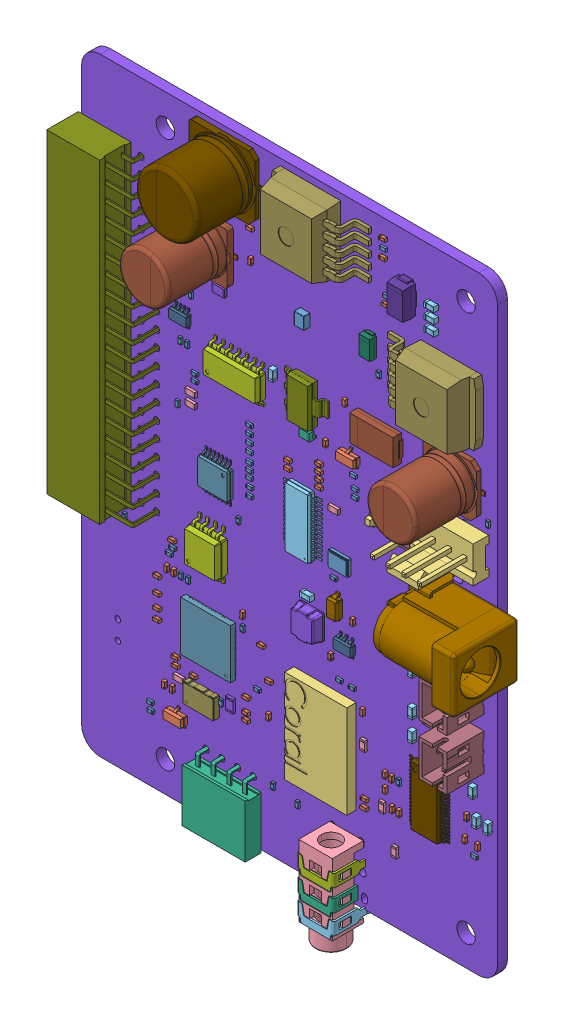
SolidWorks assembly SJ-201-R4v7, configuration Default. Lengths in mm.
Overall size (71.26 103.54 14.43).
363 component instances, 44 part files, 0 mates.
Components (placement in the parent):
- SJ-201-R4v7.step-1: SJ-201-R4v7.step [Default] at origin size (71.26 103.54 14.43)
  - R_0402_1005Metric.step-1: R_0402_1005Metric.step [Default] at (15.687 -22.3266 1.65) x (0 1 0) z (0 0 1) size (1 0.5 0.35)
    - SOLID.step-1: SOLID.step [Default] at origin size (1 0.5 0.35)
  - R_0402_1005Metric.step-2: R_0402_1005Metric.step [Default] at (27.2847 -44.6176 1.65) size (1 0.5 0.35)
    - SOLID.step-1: SOLID.step [Default] at origin size (1 0.5 0.35)
  - R_0402_1005Metric.step-3: R_0402_1005Metric.step [Default] at (15.6947 -42.2097 1.65) x (0 1 0) z (0 0 1) size (1 0.5 0.35)
    - SOLID.step-1: SOLID.step [Default] at origin size (1 0.5 0.35)
  - R_0402_1005Metric.step-4: R_0402_1005Metric.step [Default] at (44.2874 -41.0743 1.65) size (1 0.5 0.35)
    - SOLID.step-1: SOLID.step [Default] at origin size (1 0.5 0.35)
  - R_0402_1005Metric.step-5: R_0402_1005Metric.step [Default] at (44.2646 -39.8932 1.65) size (1 0.5 0.35)
    - SOLID.step-1: SOLID.step [Default] at origin size (1 0.5 0.35)
  - R_0402_1005Metric.step-6: R_0402_1005Metric.step [Default] at (65.6641 -34.0462 1.65) x (0 -1 0) z (0 0 1) size (1 0.5 0.35)
    - SOLID.step-1: SOLID.step [Default] at origin size (1 0.5 0.35)
  - R_0402_1005Metric.step-7: R_0402_1005Metric.step [Default] at (44.0182 -38.1229 1.65) x (-1 0 0) z (0 0 1) size (1 0.5 0.35)
    - SOLID.step-1: SOLID.step [Default] at origin size (1 0.5 0.35)
  - SOT-23.step-1: SOT-23.step [Default] at (43.528 -35.7327 1.65) x (0 1 0) z (0 0 1) size (2.5 3 1.2)
    - SOLID-0.step-1: SOLID-0.step [Default] at origin size (2.5 3 1.2)
  - FanPinHeader_1x04_P2.54mm_Vertical.step-1: FanPinHeader_1x04_P2.54mm_Vertical.step [Default] at (56.7182 -38.2803 1.65) size (10.2 5.84 13.5)
    - SOLID-1.step-1: SOLID-1.step [Default] at origin size (10.2 5.84 13.5)
  - TRS_Jack.step-1: TRS_Jack.step [Default] at (42.7177 -93.9744 7.15) size (6.81 14 8.02)
    - SOLID-2.step-1: SOLID-2.step [Default] at origin size (6.1 14 6)
    - SOLID-3.step-1: SOLID-3.step [Default] at origin size (6.81 2.8 8.02)
    - SOLID-4.step-1: SOLID-4.step [Default] at origin size (6.4 2.8 8.02)
    - SOLID-5.step-1: SOLID-5.step [Default] at origin size (6.81 2.8 8.02)
  - L_Bourns-SRN4018.step-1: L_Bourns-SRN4018.step [Default] at (37.2389 -61.8058 1.65) x (-1 0 0) z (0 0 1) size (4 4.09 1.8)
    - COMPOUND.step-1: COMPOUND.step [Default] at origin size (4 4.09 1.8)
  - DC_Power_Jack_5.5mm_x_2.1mm.step-1: DC_Power_Jack_5.5mm_x_2.1mm.step [Default] at (67.3554 -49.0848 8.15) x (0 1 0) z (1 0 0) size (9.77 14.38 14.62)
    - COMPOUND-6.step-1: COMPOUND-6.step [Default] at origin size (9.77 14.38 14.62)
  - TSOT-23-8.step-1: TSOT-23-8.step [Default] at (16.4084 -29.6037 1.65) x (0 1 0) z (0 0 1) size (2.8 2.9 0.95)
    - SOLID-7.step-1: SOLID-7.step [Default] at origin size (2.8 2.9 0.95)
  - CP_EIA-7343-15_Kemet-W.step-1: CP_EIA-7343-15_Kemet-W.step [Default] at (48.2143 -30.4648 1.65) size (7.3 4.3 1.5)
    - SOLID-8.step-1: SOLID-8.step [Default] at origin size (7.3 4.3 1.5)
  - TO-263-5_TabPin3.step-1: TO-263-5_TabPin3.step [Default] at (57.2872 -18.9281 1.65) size (15 10 4.42)
    - SOLID-9.step-1: SOLID-9.step [Default] at origin size (15 10 4.42)
  - R_0402_1005Metric.step-8: R_0402_1005Metric.step [Default] at (16.1417 -33.2232 1.65) x (0 -1 0) z (0 0 1) size (1 0.5 0.35)
    - SOLID.step-1: SOLID.step [Default] at origin size (1 0.5 0.35)
  - R_0402_1005Metric.step-9: R_0402_1005Metric.step [Default] at (17.8308 -25.9969 1.65) x (0 1 0) z (0 0 1) size (1 0.5 0.35)
    - SOLID.step-1: SOLID.step [Default] at origin size (1 0.5 0.35)
  - R_0402_1005Metric.step-10: R_0402_1005Metric.step [Default] at (15.5829 -26.0096 1.65) x (0 1 0) z (0 0 1) size (1 0.5 0.35)
    - SOLID.step-1: SOLID.step [Default] at origin size (1 0.5 0.35)
  - R_0402_1005Metric.step-11: R_0402_1005Metric.step [Default] at (17.2466 -33.2105 1.65) x (0 -1 0) z (0 0 1) size (1 0.5 0.35)
    - SOLID.step-1: SOLID.step [Default] at origin size (1 0.5 0.35)
  - R_0402_1005Metric.step-12: R_0402_1005Metric.step [Default] at (28.5496 -75.7174 1.65) x (-1 0 0) z (0 0 1) size (1 0.5 0.35)
    - SOLID.step-1: SOLID.step [Default] at origin size (1 0.5 0.35)
  - R_0402_1005Metric.step-13: R_0402_1005Metric.step [Default] at (16.6624 -26.0223 1.65) x (0 1 0) z (0 0 1) size (1 0.5 0.35)
    - SOLID.step-1: SOLID.step [Default] at origin size (1 0.5 0.35)
  - R_0402_1005Metric.step-14: R_0402_1005Metric.step [Default] at (27.2796 -43.1959 1.65) size (1 0.5 0.35)
    - SOLID.step-1: SOLID.step [Default] at origin size (1 0.5 0.35)
  - R_0402_1005Metric.step-15: R_0402_1005Metric.step [Default] at (27.2796 -41.9417 1.65) size (1 0.5 0.35)
    - SOLID.step-1: SOLID.step [Default] at origin size (1 0.5 0.35)
  - R_0402_1005Metric.step-16: R_0402_1005Metric.step [Default] at (7.1628 -62.2173 1.65) x (0 -1 0) z (0 0 1) size (1 0.5 0.35)
    - SOLID.step-1: SOLID.step [Default] at origin size (1 0.5 0.35)
  - JST_PH_B2B-PH-K_1x02_P2.00mm_Vertical.step-1: JST_PH_B2B-PH-K_1x02_P2.00mm_Vertical.step [Default] at (63.1698 -65.3796 1.65) x (0 -1 0) z (0 0 1) size (5.9 4.55 9.4)
    - SOLID-10.step-1: SOLID-10.step [Default] at origin size (5.9 4.55 9.4)
  - JST_PH_B2B-PH-K_1x02_P2.00mm_Vertical.step-2: JST_PH_B2B-PH-K_1x02_P2.00mm_Vertical.step [Default] at (63.1698 -57.15 1.65) x (0 -1 0) z (0 0 1) size (5.9 4.55 9.4)
    - SOLID-10.step-1: SOLID-10.step [Default] at origin size (5.9 4.55 9.4)
  - QFN-68-1EP_8x8mm_P0.4mm_EP5.2x5.2mm.step-1: QFN-68-1EP_8x8mm_P0.4mm_EP5.2x5.2mm.step [Default] at (20.8788 -72.3138 1.65) x (-1 0 0) z (0 0 1) size (8 8 0.87)
    - SOLID-11.step-1: SOLID-11.step [Default] at origin size (8 8 0.87)
  - R_0402_1005Metric.step-17: R_0402_1005Metric.step [Default] at (48.0974 -21.9862 1.65) x (0 1 0) z (0 0 1) size (1 0.5 0.35)
    - SOLID.step-1: SOLID.step [Default] at origin size (1 0.5 0.35)
  - CP_EIA-3216-10_Kemet-I.step-1: CP_EIA-3216-10_Kemet-I.step [Default] at (46.7766 -18.4201 1.65) x (0 -1 0) z (0 0 1) size (3.4 1.8 1.2)
    - SOLID-12.step-1: SOLID-12.step [Default] at origin size (3.4 1.8 1.2)
  - SOT-223.step-1: SOT-223.step [Default] at (36.4871 -31.0515 1.65) size (7 6.5 1.7)
    - SOLID-13.step-1: SOLID-13.step [Default] at origin size (7 6.5 1.7)
  - R_0402_1005Metric.step-18: R_0402_1005Metric.step [Default] at (14.3459 -63.8505 1.65) x (-1 0 0) z (0 0 1) size (1 0.5 0.35)
    - SOLID.step-1: SOLID.step [Default] at origin size (1 0.5 0.35)
  - R_0402_1005Metric.step-19: R_0402_1005Metric.step [Default] at (25.5016 -53.6396 1.65) x (0 1 0) z (0 0 1) size (1 0.5 0.35)
    - SOLID.step-1: SOLID.step [Default] at origin size (1 0.5 0.35)
  - LED_WS2812_PLCC6_5.0x5.0mm_P1.6mm.step-1: LED_WS2812_PLCC6_5.0x5.0mm_P1.6mm.step [Default] at (43.3502 -62.0185 -0.05) x (1 0 0) z (0 0 -1) size (5.4 5 1.85)
    - SOLID-14.step-1: SOLID-14.step [Default] at origin size (5.4 5 1.85)
  - R_0402_1005Metric.step-20: R_0402_1005Metric.step [Default] at (40.8559 -54.0131 1.65) x (-1 0 0) z (0 0 1) size (1 0.5 0.35)
    - SOLID.step-1: SOLID.step [Default] at origin size (1 0.5 0.35)
  - R_0402_1005Metric.step-21: R_0402_1005Metric.step [Default] at (18.4658 -37.7317 1.65) x (-1 0 0) z (0 0 1) size (1 0.5 0.35)
    - SOLID.step-1: SOLID.step [Default] at origin size (1 0.5 0.35)
  - R_0402_1005Metric.step-22: R_0402_1005Metric.step [Default] at (18.4658 -36.6903 1.65) size (1 0.5 0.35)
    - SOLID.step-1: SOLID.step [Default] at origin size (1 0.5 0.35)
  - TAS5806MD.step-1: TAS5806MD.step [Default] at (56.2187 -77.2141 1.65) size (6.4 9.7 1.09)
    - COMPOUND-15.step-1: COMPOUND-15.step [Default] at origin size (6.4 9.7 1.09)
  - L_Wuerth_MAPI-2010.step-1: L_Wuerth_MAPI-2010.step [Default] at (36.05 -20.15 1.65) x (0 1 0) z (0 0 1) size (2 1.6 1)
    - SOLID-16.step-1: SOLID-16.step [Default] at origin size (2 1.6 1)
  - C_0402_1005Metric.step-1: C_0402_1005Metric.step [Default] at (45.847 -83.5279 1.65) size (1 0.5 0.5)
    - SOLID-17.step-1: SOLID-17.step [Default] at origin size (1 0.5 0.5)
  - C_0402_1005Metric.step-2: C_0402_1005Metric.step [Default] at (45.8724 -82.2858 1.65) size (1 0.5 0.5)
    - SOLID-17.step-1: SOLID-17.step [Default] at origin size (1 0.5 0.5)
  - CoralTPU.step-1: CoralTPU.step [Default] at (39.2585 -77.2707 1.65) x (-1 0 0) z (0 0 1) size (10 15 1.5)
    - SOLID-18.step-1: SOLID-18.step [Default] at origin size (10 15 1.5)
  - R_0603_1608Metric.step-1: R_0603_1608Metric.step [Default] at (45.6946 -74.8284 1.65) x (0 1 0) z (0 0 1) size (1.6 0.8 0.45)
    - SOLID-19.step-1: SOLID-19.step [Default] at origin size (1.6 0.8 0.45)
  - C_0402_1005Metric.step-3: C_0402_1005Metric.step [Default] at (45.5676 -70.2564 1.65) x (0 1 0) z (0 0 1) size (1 0.5 0.5)
    - SOLID-17.step-1: SOLID-17.step [Default] at origin size (1 0.5 0.5)
  - R_0603_1608Metric.step-2: R_0603_1608Metric.step [Default] at (48.6918 -81.9531 1.65) x (0 -1 0) z (0 0 1) size (1.6 0.8 0.45)
    - SOLID-19.step-1: SOLID-19.step [Default] at origin size (1.6 0.8 0.45)
  - R_0402_1005Metric.step-23: R_0402_1005Metric.step [Default] at (51.3187 -77.2141 1.65) x (0 -1 0) z (0 0 1) size (1 0.5 0.35)
    - SOLID.step-1: SOLID.step [Default] at origin size (1 0.5 0.35)
  - C_0402_1005Metric.step-4: C_0402_1005Metric.step [Default] at (61.0108 -70.6247 1.65) size (1 0.5 0.5)
    - SOLID-17.step-1: SOLID-17.step [Default] at origin size (1 0.5 0.5)
  - C_0402_1005Metric.step-5: C_0402_1005Metric.step [Default] at (56.769 -71.1581 1.65) x (-1 0 0) z (0 0 1) size (1 0.5 0.5)
    - SOLID-17.step-1: SOLID-17.step [Default] at origin size (1 0.5 0.5)
  - C_0402_1005Metric.step-6: C_0402_1005Metric.step [Default] at (58.5089 -62.9666 1.65) x (-1 0 0) z (0 0 1) size (1 0.5 0.5)
    - SOLID-17.step-1: SOLID-17.step [Default] at origin size (1 0.5 0.5)
  - C_0402_1005Metric.step-7: C_0402_1005Metric.step [Default] at (57.2313 -54.6252 1.65) x (-1 0 0) z (0 0 1) size (1 0.5 0.5)
    - SOLID-17.step-1: SOLID-17.step [Default] at origin size (1 0.5 0.5)
  - C_0603_1608Metric.step-1: C_0603_1608Metric.step [Default] at (53.6829 -69.4436 1.65) x (0 1 0) z (0 0 1) size (1.6 0.8 0.8)
    - SOLID-20.step-1: SOLID-20.step [Default] at origin size (1.6 0.8 0.8)
  - C_0603_1608Metric.step-2: C_0603_1608Metric.step [Default] at (53.7464 -57.0865 1.65) x (0 1 0) z (0 0 1) size (1.6 0.8 0.8)
    - SOLID-20.step-1: SOLID-20.step [Default] at origin size (1.6 0.8 0.8)
  - C_0402_1005Metric.step-8: C_0402_1005Metric.step [Default] at (64.0715 -79.8195 1.65) x (0 1 0) z (0 0 1) size (1 0.5 0.5)
    - SOLID-17.step-1: SOLID-17.step [Default] at origin size (1 0.5 0.5)
  - C_0603_1608Metric.step-3: C_0603_1608Metric.step [Default] at (53.6956 -66.0908 1.65) x (0 1 0) z (0 0 1) size (1.6 0.8 0.8)
    - SOLID-20.step-1: SOLID-20.step [Default] at origin size (1.6 0.8 0.8)
  - C_0603_1608Metric.step-4: C_0603_1608Metric.step [Default] at (53.7083 -60.3123 1.65) x (0 1 0) z (0 0 1) size (1.6 0.8 0.8)
    - SOLID-20.step-1: SOLID-20.step [Default] at origin size (1.6 0.8 0.8)
  - C_0402_1005Metric.step-9: C_0402_1005Metric.step [Default] at (62.0395 -79.7965 1.65) x (0 1 0) z (0 0 1) size (1 0.5 0.5)
    - SOLID-17.step-1: SOLID-17.step [Default] at origin size (1 0.5 0.5)
  - C_0603_1608Metric.step-5: C_0603_1608Metric.step [Default] at (56.77 -9.66 1.65) x (-1 0 0) z (0 0 1) size (1.6 0.8 0.8)
    - SOLID-20.step-1: SOLID-20.step [Default] at origin size (1.6 0.8 0.8)
  - C_0603_1608Metric.step-6: C_0603_1608Metric.step [Default] at (56.75 -7.99 1.65) x (-1 0 0) z (0 0 1) size (1.6 0.8 0.8)
    - SOLID-20.step-1: SOLID-20.step [Default] at origin size (1.6 0.8 0.8)
  - C_0603_1608Metric.step-7: C_0603_1608Metric.step [Default] at (63.4365 -72.3392 1.65) x (0 -1 0) z (0 0 1) size (1.6 0.8 0.8)
    - SOLID-20.step-1: SOLID-20.step [Default] at origin size (1.6 0.8 0.8)
  - C_0603_1608Metric.step-8: C_0603_1608Metric.step [Default] at (56.76 -11.39 1.65) x (-1 0 0) z (0 0 1) size (1.6 0.8 0.8)
    - SOLID-20.step-1: SOLID-20.step [Default] at origin size (1.6 0.8 0.8)
  - C_0402_1005Metric.step-10: C_0402_1005Metric.step [Default] at (49.1787 -79.3091 1.65) x (0 1 0) z (0 0 1) size (1 0.5 0.5)
    - SOLID-17.step-1: SOLID-17.step [Default] at origin size (1 0.5 0.5)
  - C_0402_1005Metric.step-11: C_0402_1005Metric.step [Default] at (62.324 -76.5429 1.65) x (0 1 0) z (0 0 1) size (1 0.5 0.5)
    - SOLID-17.step-1: SOLID-17.step [Default] at origin size (1 0.5 0.5)
  - C_0603_1608Metric.step-9: C_0603_1608Metric.step [Default] at (65.8537 -76.2041 1.65) x (0 -1 0) z (0 0 1) size (1.6 0.8 0.8)
    - SOLID-20.step-1: SOLID-20.step [Default] at origin size (1.6 0.8 0.8)
  - C_0603_1608Metric.step-10: C_0603_1608Metric.step [Default] at (64.0287 -76.2041 1.65) x (0 -1 0) z (0 0 1) size (1.6 0.8 0.8)
    - SOLID-20.step-1: SOLID-20.step [Default] at origin size (1.6 0.8 0.8)
  - C_0402_1005Metric.step-12: C_0402_1005Metric.step [Default] at (51.4187 -81.4141 1.65) x (0 -1 0) z (0 0 1) size (1 0.5 0.5)
    - SOLID-17.step-1: SOLID-17.step [Default] at origin size (1 0.5 0.5)
  - C_0402_1005Metric.step-13: C_0402_1005Metric.step [Default] at (50.2387 -77.2091 1.65) x (0 -1 0) z (0 0 1) size (1 0.5 0.5)
    - SOLID-17.step-1: SOLID-17.step [Default] at origin size (1 0.5 0.5)
  - LED_WS2812_PLCC6_5.0x5.0mm_P1.6mm.step-2: LED_WS2812_PLCC6_5.0x5.0mm_P1.6mm.step [Default] at (35.8318 -35.3485 -0.05) x (1 0 0) z (0 0 -1) size (5.4 5 1.85)
    - SOLID-14.step-1: SOLID-14.step [Default] at origin size (5.4 5 1.85)
  - LED_WS2812_PLCC6_5.0x5.0mm_P1.6mm.step-3: LED_WS2812_PLCC6_5.0x5.0mm_P1.6mm.step [Default] at (43.2994 -36.0089 -0.05) x (1 0 0) z (0 0 -1) size (5.4 5 1.85)
    - SOLID-14.step-1: SOLID-14.step [Default] at origin size (5.4 5 1.85)
  - LED_WS2812_PLCC6_5.0x5.0mm_P1.6mm.step-4: LED_WS2812_PLCC6_5.0x5.0mm_P1.6mm.step [Default] at (47.6682 -42.2065 -0.05) x (1 0 0) z (0 0 -1) size (5.4 5 1.85)
    - SOLID-14.step-1: SOLID-14.step [Default] at origin size (5.4 5 1.85)
  - LED_WS2812_PLCC6_5.0x5.0mm_P1.6mm.step-5: LED_WS2812_PLCC6_5.0x5.0mm_P1.6mm.step [Default] at (50.8178 -49.0137 -0.05) x (1 0 0) z (0 0 -1) size (5.4 5 1.85)
    - SOLID-14.step-1: SOLID-14.step [Default] at origin size (5.4 5 1.85)
  - LED_WS2812_PLCC6_5.0x5.0mm_P1.6mm.step-6: LED_WS2812_PLCC6_5.0x5.0mm_P1.6mm.step [Default] at (47.719 -55.8209 -0.05) x (1 0 0) z (0 0 -1) size (5.4 5 1.85)
    - SOLID-14.step-1: SOLID-14.step [Default] at origin size (5.4 5 1.85)
  - LED_WS2812_PLCC6_5.0x5.0mm_P1.6mm.step-7: LED_WS2812_PLCC6_5.0x5.0mm_P1.6mm.step [Default] at (35.8318 -62.6281 -0.05) x (1 0 0) z (0 0 -1) size (5.4 5 1.85)
    - SOLID-14.step-1: SOLID-14.step [Default] at origin size (5.4 5 1.85)
  - LED_WS2812_PLCC6_5.0x5.0mm_P1.6mm.step-8: LED_WS2812_PLCC6_5.0x5.0mm_P1.6mm.step [Default] at (28.3642 -61.9677 -0.05) x (1 0 0) z (0 0 -1) size (5.4 5 1.85)
    - SOLID-14.step-1: SOLID-14.step [Default] at origin size (5.4 5 1.85)
  - LED_WS2812_PLCC6_5.0x5.0mm_P1.6mm.step-9: LED_WS2812_PLCC6_5.0x5.0mm_P1.6mm.step [Default] at (23.9446 -55.9225 -0.05) x (1 0 0) z (0 0 -1) size (5.4 5 1.85)
    - SOLID-14.step-1: SOLID-14.step [Default] at origin size (5.4 5 1.85)
  - LED_WS2812_PLCC6_5.0x5.0mm_P1.6mm.step-10: LED_WS2812_PLCC6_5.0x5.0mm_P1.6mm.step [Default] at (20.8458 -49.0645 -0.05) x (1 0 0) z (0 0 -1) size (5.4 5 1.85)
    - SOLID-14.step-1: SOLID-14.step [Default] at origin size (5.4 5 1.85)
  - LED_WS2812_PLCC6_5.0x5.0mm_P1.6mm.step-11: LED_WS2812_PLCC6_5.0x5.0mm_P1.6mm.step [Default] at (28.3134 -36.1105 -0.05) x (1 0 0) z (0 0 -1) size (5.4 5 1.85)
    - SOLID-14.step-1: SOLID-14.step [Default] at origin size (5.4 5 1.85)
  - LED_WS2812_PLCC6_5.0x5.0mm_P1.6mm.step-12: LED_WS2812_PLCC6_5.0x5.0mm_P1.6mm.step [Default] at (23.9954 -42.2065 -0.05) x (1 0 0) z (0 0 -1) size (5.4 5 1.85)
    - SOLID-14.step-1: SOLID-14.step [Default] at origin size (5.4 5 1.85)
  - R_0603_1608Metric.step-3: R_0603_1608Metric.step [Default] at (50.7441 -87.1931 1.65) x (0 -1 0) z (0 0 1) size (1.6 0.8 0.45)
    - SOLID-19.step-1: SOLID-19.step [Default] at origin size (1.6 0.8 0.45)
  - R_0603_1608Metric.step-4: R_0603_1608Metric.step [Default] at (4.425 -27.75 -0.05) x (-1 0 0) z (0 0 -1) size (1.6 0.8 0.45)
    - SOLID-19.step-1: SOLID-19.step [Default] at origin size (1.6 0.8 0.45)
  - R_0603_1608Metric.step-5: R_0603_1608Metric.step [Default] at (15.9207 -49.3624 -0.05) x (0 1 0) z (0 0 -1) size (1.6 0.8 0.45)
    - SOLID-19.step-1: SOLID-19.step [Default] at origin size (1.6 0.8 0.45)
  - R_0603_1608Metric.step-6: R_0603_1608Metric.step [Default] at (17.907 -41.1607 1.65) size (1.6 0.8 0.45)
    - SOLID-19.step-1: SOLID-19.step [Default] at origin size (1.6 0.8 0.45)
  - R_0603_1608Metric.step-7: R_0603_1608Metric.step [Default] at (17.9158 -39.5478 1.65) size (1.6 0.8 0.45)
    - SOLID-19.step-1: SOLID-19.step [Default] at origin size (1.6 0.8 0.45)
  - R_0603_1608Metric.step-8: R_0603_1608Metric.step [Default] at (4.425 -31.1 -0.05) x (1 0 0) z (0 0 -1) size (1.6 0.8 0.45)
    - SOLID-19.step-1: SOLID-19.step [Default] at origin size (1.6 0.8 0.45)
  - SOT-23.step-2: SOT-23.step [Default] at (52.5399 -37.8587 1.65) x (0 -1 0) z (0 0 1) size (2.5 3 1.2)
    - SOLID-0.step-1: SOLID-0.step [Default] at origin size (2.5 3 1.2)
  - PinSocket_1x04_P2.54mm_Horizontal.step-1: PinSocket_1x04_P2.54mm_Horizontal.step [Default] at (20.05 -88.4 1.65) x (0 1 0) z (0 0 1) size (10.13 10.16 5.84)
    - SOLID-21.step-1: SOLID-21.step [Default] at origin size (10.13 10.16 5.84)
  - SOIC-8_5.275x5.275mm_P1.27mm.step-1: SOIC-8_5.275x5.275mm_P1.27mm.step [Default] at (21.0998 -59.7179 1.65) x (0 1 0) z (0 0 1) size (7.9 5.28 2.06)
    - SOLID-22.step-1: SOLID-22.step [Default] at origin size (7.9 5.28 2.06)
  - R_0805_2012Metric.step-1: R_0805_2012Metric.step [Default] at (22.4663 -22.987 1.65) x (-1 0 0) z (0 0 1) size (2 1.2 0.45)
    - SOLID-23.step-1: SOLID-23.step [Default] at origin size (2 1.2 0.45)
  - R_0402_1005Metric.step-24: R_0402_1005Metric.step [Default] at (16.278 -65.9816 1.65) x (0 1 0) z (0 0 1) size (1 0.5 0.35)
    - SOLID.step-1: SOLID.step [Default] at origin size (1 0.5 0.35)
  - D_SOD-123.step-1: D_SOD-123.step [Default] at (41.4376 -57.6783 1.65) x (0 1 0) z (0 0 1) size (3.8 1.6 1.25)
    - SOLID-24.step-1: SOLID-24.step [Default] at origin size (3.8 1.6 1.25)
  - C_0402_1005Metric.step-14: C_0402_1005Metric.step [Default] at (43.975 -58.4657 1.65) x (0 -1 0) z (0 0 1) size (1 0.5 0.5)
    - SOLID-17.step-1: SOLID-17.step [Default] at origin size (1 0.5 0.5)
  - C_0402_1005Metric.step-15: C_0402_1005Metric.step [Default] at (40.4241 -65.0723 1.65) x (0 -1 0) z (0 0 1) size (1 0.5 0.5)
    - SOLID-17.step-1: SOLID-17.step [Default] at origin size (1 0.5 0.5)
  - C_0603_1608Metric.step-11: C_0603_1608Metric.step [Default] at (36.7716 -58.3819 1.65) size (1.6 0.8 0.8)
    - SOLID-20.step-1: SOLID-20.step [Default] at origin size (1.6 0.8 0.8)
  - R_0402_1005Metric.step-25: R_0402_1005Metric.step [Default] at (41.7449 -67.8104 1.65) size (1 0.5 0.35)
    - SOLID.step-1: SOLID.step [Default] at origin size (1 0.5 0.35)
  - R_0402_1005Metric.step-26: R_0402_1005Metric.step [Default] at (43.8125 -67.8282 1.65) x (-1 0 0) z (0 0 1) size (1 0.5 0.35)
    - SOLID.step-1: SOLID.step [Default] at origin size (1 0.5 0.35)
  - TSOT-23-6.step-1: TSOT-23-6.step [Default] at (42.832 -62.4281 1.65) x (0 1 0) z (0 0 1) size (2.8 2.9 0.95)
    - SOLID-25.step-1: SOLID-25.step [Default] at origin size (2.8 2.9 0.95)
  - CP_Elec_8x10.5.step-1: CP_Elec_8x10.5.step [Default] at (60.3656 -30.2311 1.65) x (-1 0 0) z (0 0 1) size (10.73 10.93 10.5)
    - SOLID-26.step-1: SOLID-26.step [Default] at origin size (10.73 10.93 10.5)
  - CP_Elec_8x10.5.step-2: CP_Elec_8x10.5.step [Default] at (20.4749 -17.2568 1.65) size (10.73 10.93 10.5)
    - SOLID-26.step-1: SOLID-26.step [Default] at origin size (10.73 10.93 10.5)
  - R_0603_1608Metric.step-9: R_0603_1608Metric.step [Default] at (16 -80.4 1.65) x (-1 0 0) z (0 0 1) size (1.6 0.8 0.45)
    - SOLID-19.step-1: SOLID-19.step [Default] at origin size (1.6 0.8 0.45)
  - Oscillator_SMD_EuroQuartz_XO53-4Pin_5.0x3.2mm.step-1: Oscillator_SMD_EuroQuartz_XO53-4Pin_5.0x3.2mm.step [Default] at (19.7732 -81.3418 1.65) size (5 3.2 1)
    - SOLID-27.step-1: SOLID-27.step [Default] at origin size (5 3.2 1)
  - R_1206_3216Metric.step-1: R_1206_3216Metric.step [Default] at (52.578 -42.3672 1.65) x (0 1 0) z (0 0 1) size (3.2 1.6 0.55)
    - SOLID-28.step-1: SOLID-28.step [Default] at origin size (3.2 1.6 0.55)
  - R_1206_3216Metric.step-2: R_1206_3216Metric.step [Default] at (56.9976 -66.04 1.65) x (-1 0 0) z (0 0 1) size (3.2 1.6 0.55)
    - SOLID-28.step-1: SOLID-28.step [Default] at origin size (3.2 1.6 0.55)
  - R_1206_3216Metric.step-3: R_1206_3216Metric.step [Default] at (56.9976 -69.342 1.65) x (-1 0 0) z (0 0 1) size (3.2 1.6 0.55)
    - SOLID-28.step-1: SOLID-28.step [Default] at origin size (3.2 1.6 0.55)
  - R_1206_3216Metric.step-4: R_1206_3216Metric.step [Default] at (57.0357 -60.579 1.65) x (-1 0 0) z (0 0 1) size (3.2 1.6 0.55)
    - SOLID-28.step-1: SOLID-28.step [Default] at origin size (3.2 1.6 0.55)
  - R_1206_3216Metric.step-5: R_1206_3216Metric.step [Default] at (56.9976 -57.2135 1.65) x (-1 0 0) z (0 0 1) size (3.2 1.6 0.55)
    - SOLID-28.step-1: SOLID-28.step [Default] at origin size (3.2 1.6 0.55)
  - TSSOP-14_4.4x5mm_P0.65mm.step-1: TSSOP-14_4.4x5mm_P0.65mm.step [Default] at (22.1234 -49.2125 1.65) x (0 -1 0) z (0 0 1) size (6.4 5 1)
    - SOLID-29.step-1: SOLID-29.step [Default] at origin size (6.4 5 1)
  - User_Library-WM7121PE.step-1: User_Library-WM7121PE.step [Default] at (24.8082 -13.9141 -0.05) x (1 0 0) z (0 1 0) size (3.76 1.1 2.95)
    - SOLID-30.step-1: SOLID-30.step [Default] at origin size (3.76 1.1 2.95)
  - User_Library-WM7121PE.step-2: User_Library-WM7121PE.step [Default] at (24.8082 -83.7641 -0.05) x (1 0 0) z (0 1 0) size (3.76 1.1 2.95)
    - SOLID-30.step-1: SOLID-30.step [Default] at origin size (3.76 1.1 2.95)
  - R_0805_2012Metric.step-2: R_0805_2012Metric.step [Default] at (24.2631 -79.9121 1.65) x (0 1 0) z (0 0 1) size (2 1.2 0.45)
    - SOLID-23.step-1: SOLID-23.step [Default] at origin size (2 1.2 0.45)
  - R_0603_1608Metric.step-10: R_0603_1608Metric.step [Default] at (40.9499 -44.3306 1.65) size (1.6 0.8 0.45)
    - SOLID-19.step-1: SOLID-19.step [Default] at origin size (1.6 0.8 0.45)
  - PinSocket_2x20_P2.54mm_Horizontal.step-1: PinSocket_2x20_P2.54mm_Horizontal.step [Default] at (12.0929 -10.9779 1.65) size (12.67 50.8 7.98)
    - SOLID-31.step-1: SOLID-31.step [Default] at origin size (12.67 50.8 7.98)
  - D_SMA.step-1: D_SMA.step [Default] at (52.725 -8.6 1.65) x (0 -1 0) z (0 0 1) size (5 2.7 2.22)
    - SOLID-32.step-1: SOLID-32.step [Default] at origin size (5 2.7 2.22)
  - TO-263-5_TabPin3.step-2: TO-263-5_TabPin3.step [Default] at (39.25 -6 1.65) x (-1 0 0) z (0 0 1) size (15 10 4.42)
    - SOLID-9.step-1: SOLID-9.step [Default] at origin size (15 10 4.42)
  - R_0402_1005Metric.step-27: R_0402_1005Metric.step [Default] at (49.3108 -10.461 1.65) x (-1 0 0) z (0 0 1) size (1 0.5 0.35)
    - SOLID.step-1: SOLID.step [Default] at origin size (1 0.5 0.35)
  - C_0402_1005Metric.step-16: C_0402_1005Metric.step [Default] at (49.3108 -11.611 1.65) x (-1 0 0) z (0 0 1) size (1 0.5 0.5)
    - SOLID-17.step-1: SOLID-17.step [Default] at origin size (1 0.5 0.5)
  - C_0402_1005Metric.step-17: C_0402_1005Metric.step [Default] at (48.85 -2.6 1.65) size (1 0.5 0.5)
    - SOLID-17.step-1: SOLID-17.step [Default] at origin size (1 0.5 0.5)
  - CP_Elec_10x10.step-1: CP_Elec_10x10.step [Default] at (23.65 -5.75 1.65) x (-1 0 0) z (0 0 1) size (13.47 13.66 10)
    - SOLID-33.step-1: SOLID-33.step [Default] at origin size (13.47 13.66 10)
  - C_0603_1608Metric.step-12: C_0603_1608Metric.step [Default] at (31.242 -30.226 1.65) x (0 1 0) z (0 0 1) size (1.6 0.8 0.8)
    - SOLID-20.step-1: SOLID-20.step [Default] at origin size (1.6 0.8 0.8)
  - C_0402_1005Metric.step-18: C_0402_1005Metric.step [Default] at (42.7101 -28.5242 1.65) x (0 -1 0) z (0 0 1) size (1 0.5 0.5)
    - SOLID-17.step-1: SOLID-17.step [Default] at origin size (1 0.5 0.5)
  - C_0402_1005Metric.step-19: C_0402_1005Metric.step [Default] at (52.4916 -45.6489 1.65) size (1 0.5 0.5)
    - SOLID-17.step-1: SOLID-17.step [Default] at origin size (1 0.5 0.5)
  - C_0402_1005Metric.step-20: C_0402_1005Metric.step [Default] at (50.2987 -81.4091 1.65) x (0 -1 0) z (0 0 1) size (1 0.5 0.5)
    - SOLID-17.step-1: SOLID-17.step [Default] at origin size (1 0.5 0.5)
  - R_0402_1005Metric.step-28: R_0402_1005Metric.step [Default] at (63.5281 -81.5035 1.65) x (-1 0 0) z (0 0 1) size (1 0.5 0.35)
    - SOLID.step-1: SOLID.step [Default] at origin size (1 0.5 0.35)
  - R_0402_1005Metric.step-29: R_0402_1005Metric.step [Default] at (27.2593 -39.4443 1.65) size (1 0.5 0.35)
    - SOLID.step-1: SOLID.step [Default] at origin size (1 0.5 0.35)
  - R_0402_1005Metric.step-30: R_0402_1005Metric.step [Default] at (27.2593 -40.6984 1.65) size (1 0.5 0.35)
    - SOLID.step-1: SOLID.step [Default] at origin size (1 0.5 0.35)
  - Crystal_SMD_3225-4Pin_3.2x2.5mm.step-1: Crystal_SMD_3225-4Pin_3.2x2.5mm.step [Default] at (41.8389 -51.3537 1.65) size (3.2 2.5 0.64)
    - SOLID-34.step-1: SOLID-34.step [Default] at origin size (3.2 2.5 0.64)
  - SW_SPDT_PCM12.step-1: SW_SPDT_PCM12.step [Default] at (6.1849 -78.8822 -0.05) x (0 1 0) z (0 0 -1) size (7.7 5 2)
    - SOLID-35.step-1: SOLID-35.step [Default] at origin size (7.7 5 2)
  - R_0402_1005Metric.step-31: R_0402_1005Metric.step [Default] at (27.2745 -45.7454 1.65) x (-1 0 0) z (0 0 1) size (1 0.5 0.35)
    - SOLID.step-1: SOLID.step [Default] at origin size (1 0.5 0.35)
  - R_0402_1005Metric.step-32: R_0402_1005Metric.step [Default] at (27.2745 -46.802 1.65) size (1 0.5 0.35)
    - SOLID.step-1: SOLID.step [Default] at origin size (1 0.5 0.35)
  - R_0402_1005Metric.step-33: R_0402_1005Metric.step [Default] at (48.6054 -42.1437 1.65) x (0 1 0) z (0 0 1) size (1 0.5 0.35)
    - SOLID.step-1: SOLID.step [Default] at origin size (1 0.5 0.35)
  - LED_0603_1608Metric.step-1: LED_0603_1608Metric.step [Default] at (47.1983 -42.6364 1.65) x (0 1 0) z (0 0 1) size (1.6 0.8 1.1)
    - SOLID-36.step-1: SOLID-36.step [Default] at origin size (1.6 0.8 1.1)
  - C_0402_1005Metric.step-21: C_0402_1005Metric.step [Default] at (38.5318 -40.2759 1.65) size (1 0.5 0.5)
    - SOLID-17.step-1: SOLID-17.step [Default] at origin size (1 0.5 0.5)
  - C_0402_1005Metric.step-22: C_0402_1005Metric.step [Default] at (26.7827 -79.7546 1.65) x (-1 0 0) z (0 0 1) size (1 0.5 0.5)
    - SOLID-17.step-1: SOLID-17.step [Default] at origin size (1 0.5 0.5)
  - C_0402_1005Metric.step-23: C_0402_1005Metric.step [Default] at (27.5336 -16.3703 1.65) x (0 -1 0) z (0 0 1) size (1 0.5 0.5)
    - SOLID-17.step-1: SOLID-17.step [Default] at origin size (1 0.5 0.5)
  - C_0402_1005Metric.step-24: C_0402_1005Metric.step [Default] at (26.7827 -80.8316 1.65) x (-1 0 0) z (0 0 1) size (1 0.5 0.5)
    - SOLID-17.step-1: SOLID-17.step [Default] at origin size (1 0.5 0.5)
  - C_0402_1005Metric.step-25: C_0402_1005Metric.step [Default] at (27.4193 -11.8745 1.65) size (1 0.5 0.5)
    - SOLID-17.step-1: SOLID-17.step [Default] at origin size (1 0.5 0.5)
  - C_0402_1005Metric.step-26: C_0402_1005Metric.step [Default] at (14.8946 -61.6991 1.65) size (1 0.5 0.5)
    - SOLID-17.step-1: SOLID-17.step [Default] at origin size (1 0.5 0.5)
  - C_0402_1005Metric.step-27: C_0402_1005Metric.step [Default] at (30.4698 -73.5787 1.65) size (1 0.5 0.5)
    - SOLID-17.step-1: SOLID-17.step [Default] at origin size (1 0.5 0.5)
  - C_0402_1005Metric.step-28: C_0402_1005Metric.step [Default] at (29.2456 -69.1794 1.65) size (1 0.5 0.5)
    - SOLID-17.step-1: SOLID-17.step [Default] at origin size (1 0.5 0.5)
  - C_0402_1005Metric.step-29: C_0402_1005Metric.step [Default] at (26.8224 -77.6351 1.65) size (1 0.5 0.5)
    - SOLID-17.step-1: SOLID-17.step [Default] at origin size (1 0.5 0.5)
  - C_0402_1005Metric.step-30: C_0402_1005Metric.step [Default] at (15.1519 -65.9816 1.65) x (0 1 0) z (0 0 1) size (1 0.5 0.5)
    - SOLID-17.step-1: SOLID-17.step [Default] at origin size (1 0.5 0.5)
  - C_0402_1005Metric.step-31: C_0402_1005Metric.step [Default] at (18.3261 -78.8924 1.65) size (1 0.5 0.5)
    - SOLID-17.step-1: SOLID-17.step [Default] at origin size (1 0.5 0.5)
  - C_0402_1005Metric.step-32: C_0402_1005Metric.step [Default] at (15.4596 -77.6828 1.65) x (-1 0 0) z (0 0 1) size (1 0.5 0.5)
    - SOLID-17.step-1: SOLID-17.step [Default] at origin size (1 0.5 0.5)
  - C_0402_1005Metric.step-33: C_0402_1005Metric.step [Default] at (12.4968 -70.2818 1.65) x (-1 0 0) z (0 0 1) size (1 0.5 0.5)
    - SOLID-17.step-1: SOLID-17.step [Default] at origin size (1 0.5 0.5)
  - C_0402_1005Metric.step-34: C_0402_1005Metric.step [Default] at (30.4089 -78.4809 1.65) x (0 -1 0) z (0 0 1) size (1 0.5 0.5)
    - SOLID-17.step-1: SOLID-17.step [Default] at origin size (1 0.5 0.5)
  - C_0402_1005Metric.step-35: C_0402_1005Metric.step [Default] at (12.4746 -73.9377 1.65) x (-1 0 0) z (0 0 1) size (1 0.5 0.5)
    - SOLID-17.step-1: SOLID-17.step [Default] at origin size (1 0.5 0.5)
  - C_0402_1005Metric.step-36: C_0402_1005Metric.step [Default] at (12.5 -72.35 1.65) x (-1 0 0) z (0 0 1) size (1 0.5 0.5)
    - SOLID-17.step-1: SOLID-17.step [Default] at origin size (1 0.5 0.5)
  - C_0402_1005Metric.step-37: C_0402_1005Metric.step [Default] at (14.9 -82.375 1.65) x (0 -1 0) z (0 0 1) size (1 0.5 0.5)
    - SOLID-17.step-1: SOLID-17.step [Default] at origin size (1 0.5 0.5)
  - C_0402_1005Metric.step-38: C_0402_1005Metric.step [Default] at (14.0259 -65.9816 1.65) x (0 1 0) z (0 0 1) size (1 0.5 0.5)
    - SOLID-17.step-1: SOLID-17.step [Default] at origin size (1 0.5 0.5)
  - C_0402_1005Metric.step-39: C_0402_1005Metric.step [Default] at (26.2433 -66.3854 1.65) x (0 1 0) z (0 0 1) size (1 0.5 0.5)
    - SOLID-17.step-1: SOLID-17.step [Default] at origin size (1 0.5 0.5)
  - C_0402_1005Metric.step-40: C_0402_1005Metric.step [Default] at (13.65 -82.375 1.65) x (0 -1 0) z (0 0 1) size (1 0.5 0.5)
    - SOLID-17.step-1: SOLID-17.step [Default] at origin size (1 0.5 0.5)
  - C_0402_1005Metric.step-41: C_0402_1005Metric.step [Default] at (15.4596 -78.8868 1.65) x (-1 0 0) z (0 0 1) size (1 0.5 0.5)
    - SOLID-17.step-1: SOLID-17.step [Default] at origin size (1 0.5 0.5)
  - C_0402_1005Metric.step-42: C_0402_1005Metric.step [Default] at (12.4746 -67.8569 1.65) x (-1 0 0) z (0 0 1) size (1 0.5 0.5)
    - SOLID-17.step-1: SOLID-17.step [Default] at origin size (1 0.5 0.5)
  - C_0402_1005Metric.step-43: C_0402_1005Metric.step [Default] at (38.5318 -39.1795 1.65) x (-1 0 0) z (0 0 1) size (1 0.5 0.5)
    - SOLID-17.step-1: SOLID-17.step [Default] at origin size (1 0.5 0.5)
  - C_0402_1005Metric.step-44: C_0402_1005Metric.step [Default] at (38.5318 -42.4688 1.65) size (1 0.5 0.5)
    - SOLID-17.step-1: SOLID-17.step [Default] at origin size (1 0.5 0.5)
  - C_0402_1005Metric.step-45: C_0402_1005Metric.step [Default] at (38.5318 -41.3724 1.65) x (-1 0 0) z (0 0 1) size (1 0.5 0.5)
    - SOLID-17.step-1: SOLID-17.step [Default] at origin size (1 0.5 0.5)
  - C_0402_1005Metric.step-46: C_0402_1005Metric.step [Default] at (33.528 -42.3621 1.65) x (-1 0 0) z (0 0 1) size (1 0.5 0.5)
    - SOLID-17.step-1: SOLID-17.step [Default] at origin size (1 0.5 0.5)
  - C_0402_1005Metric.step-47: C_0402_1005Metric.step [Default] at (33.528 -41.2064 1.65) size (1 0.5 0.5)
    - SOLID-17.step-1: SOLID-17.step [Default] at origin size (1 0.5 0.5)
  - C_0402_1005Metric.step-48: C_0402_1005Metric.step [Default] at (39.5859 -35.7632 1.65) x (0 1 0) z (0 0 1) size (1 0.5 0.5)
    - SOLID-17.step-1: SOLID-17.step [Default] at origin size (1 0.5 0.5)
  - C_0402_1005Metric.step-49: C_0402_1005Metric.step [Default] at (48.85 -5.3 1.65) x (-1 0 0) z (0 0 1) size (1 0.5 0.5)
    - SOLID-17.step-1: SOLID-17.step [Default] at origin size (1 0.5 0.5)
  - R_0402_1005Metric.step-34: R_0402_1005Metric.step [Default] at (54.2671 -34.3408 1.65) size (1 0.5 0.35)
    - SOLID.step-1: SOLID.step [Default] at origin size (1 0.5 0.35)
  - R_0402_1005Metric.step-35: R_0402_1005Metric.step [Default] at (11.3792 -87.2617 1.65) size (1 0.5 0.35)
    - SOLID.step-1: SOLID.step [Default] at origin size (1 0.5 0.35)
  - R_0402_1005Metric.step-36: R_0402_1005Metric.step [Default] at (11.3157 -86.0806 1.65) size (1 0.5 0.35)
    - SOLID.step-1: SOLID.step [Default] at origin size (1 0.5 0.35)
  - R_0402_1005Metric.step-37: R_0402_1005Metric.step [Default] at (21.0566 -11.9761 1.65) size (1 0.5 0.35)
    - SOLID.step-1: SOLID.step [Default] at origin size (1 0.5 0.35)
  - R_0402_1005Metric.step-38: R_0402_1005Metric.step [Default] at (23.6982 -11.9761 1.65) x (-1 0 0) z (0 0 1) size (1 0.5 0.35)
    - SOLID.step-1: SOLID.step [Default] at origin size (1 0.5 0.35)
  - R_0402_1005Metric.step-39: R_0402_1005Metric.step [Default] at (26.1849 -68.3463 1.65) x (0 -1 0) z (0 0 1) size (1 0.5 0.35)
    - SOLID.step-1: SOLID.step [Default] at origin size (1 0.5 0.35)
  - R_0402_1005Metric.step-40: R_0402_1005Metric.step [Default] at (35.0393 -88.4809 1.65) x (0 -1 0) z (0 0 1) size (1 0.5 0.35)
    - SOLID.step-1: SOLID.step [Default] at origin size (1 0.5 0.35)
  - R_0402_1005Metric.step-41: R_0402_1005Metric.step [Default] at (31.0794 -87.8942 1.65) x (0 -1 0) z (0 0 1) size (1 0.5 0.35)
    - SOLID.step-1: SOLID.step [Default] at origin size (1 0.5 0.35)
  - R_0402_1005Metric.step-42: R_0402_1005Metric.step [Default] at (17.4041 -65.9816 1.65) x (0 -1 0) z (0 0 1) size (1 0.5 0.35)
    - SOLID.step-1: SOLID.step [Default] at origin size (1 0.5 0.35)
  - R_0402_1005Metric.step-43: R_0402_1005Metric.step [Default] at (22.7232 -80.4418 1.65) x (0 -1 0) z (0 0 1) size (1 0.5 0.35)
    - SOLID.step-1: SOLID.step [Default] at origin size (1 0.5 0.35)
  - R_0402_1005Metric.step-44: R_0402_1005Metric.step [Default] at (27.3126 -49.3573 1.65) size (1 0.5 0.35)
    - SOLID.step-1: SOLID.step [Default] at origin size (1 0.5 0.35)
  - R_0402_1005Metric.step-45: R_0402_1005Metric.step [Default] at (14.9022 -62.7685 1.65) x (-1 0 0) z (0 0 1) size (1 0.5 0.35)
    - SOLID.step-1: SOLID.step [Default] at origin size (1 0.5 0.35)
  - R_0402_1005Metric.step-46: R_0402_1005Metric.step [Default] at (27.3126 -48.0873 1.65) size (1 0.5 0.35)
    - SOLID.step-1: SOLID.step [Default] at origin size (1 0.5 0.35)
  - R_0402_1005Metric.step-47: R_0402_1005Metric.step [Default] at (48.85 -4.05 1.65) x (-1 0 0) z (0 0 1) size (1 0.5 0.35)
    - SOLID.step-1: SOLID.step [Default] at origin size (1 0.5 0.35)
  - SOT-23.step-3: SOT-23.step [Default] at (15.748 -85.7758 1.65) x (0 1 0) z (0 0 1) size (2.5 3 1.2)
    - SOLID-0.step-1: SOLID-0.step [Default] at origin size (2.5 3 1.2)
  - SW_SPST_TL3342.step-1: SW_SPST_TL3342.step [Default] at (35.6108 -48.9934 -0.05) x (1 0 0) z (0 0 -1) size (6.4 5.2 1.54)
    - SOLID-37.step-1: SOLID-37.step [Default] at origin size (6.4 5.2 1.54)
  - SW_SPST_TL3342.step-2: SW_SPST_TL3342.step [Default] at (4.478 -49 -0.05) x (0 1 0) z (0 0 -1) size (6.4 5.2 1.54)
    - SOLID-37.step-1: SOLID-37.step [Default] at origin size (6.4 5.2 1.54)
  - SW_SPST_TL3342.step-3: SW_SPST_TL3342.step [Default] at (4.4729 -18.7401 -0.05) x (0 1 0) z (0 0 -1) size (6.4 5.2 1.54)
    - SOLID-37.step-1: SOLID-37.step [Default] at origin size (6.4 5.2 1.54)
  - SSOP-28_3.9x9.9mm_P0.635mm.step-1: SSOP-28_3.9x9.9mm_P0.635mm.step [Default] at (35.7429 -48.4581 1.65) x (-1 0 0) z (0 0 1) size (6.2 9.9 1.1)
    - SOLID-38.step-1: SOLID-38.step [Default] at origin size (6.2 9.9 1.1)
  - D_SOD-323F.step-1: D_SOD-323F.step [Default] at (36.6141 -35.9054 1.65) x (-1 0 0) z (0 0 1) size (2.5 1.25 0.73)
    - SOLID-39.step-1: SOLID-39.step [Default] at origin size (2.5 1.25 0.73)
  - C_0402_1005Metric.step-50: C_0402_1005Metric.step [Default] at (49.1687 -77.2141 1.65) x (0 -1 0) z (0 0 1) size (1 0.5 0.5)
    - SOLID-17.step-1: SOLID-17.step [Default] at origin size (1 0.5 0.5)
  - SOIC-14_3.9x8.7mm_P1.27mm.step-1: SOIC-14_3.9x8.7mm_P1.27mm.step [Default] at (25.5524 -32.7787 1.65) x (0 1 0) z (0 0 1) size (6 8.7 1.75)
    - SOLID-40.step-1: SOLID-40.step [Default] at origin size (6 8.7 1.75)
  - COMPOUND-41.step-1: COMPOUND-41.step [Default] at origin size (67 98 1.6)
